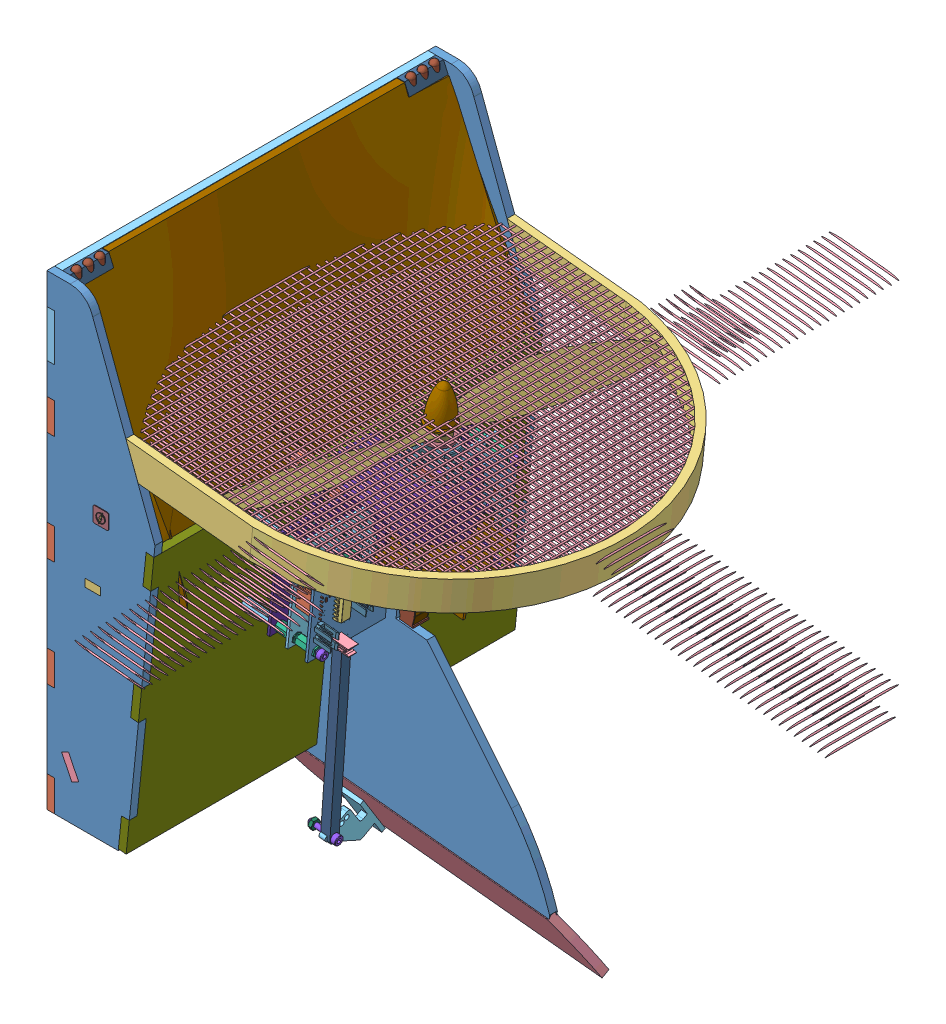
SolidWorks assembly AssTotaleSimu8, configuration Défaut. Lengths in mm. (continued)
Components (placement in the parent): (continued)
- AssStructSimu-1: AssStructSimu [Défaut] at (-125.7658 -1.8483 624.6548) x (1 0 0) z (0 0 -1) size (253.25 324.59 251.6) (continued)
  - AssCarte-1: AssCarte [Défaut] at (-42.8534 32.2132 302.028) x (-0.101852 0.9948 0) z (0.9948 0.101852 0) size (67.15 130.57 98.45) (continued)
    - carte_onduleur_v4-1: carte_onduleur_v4 [Défaut] at (-25.7639 0.8332 112.9379) size (66.52 130.57 82.34) (continued)
      - CARTE_CMD-1: CARTE_CMD [Défaut] at (25 57.2 0.803) size (60.1 130 26.71) (continued)
        - Open CASCADE STEP translator 6.8 1.20.1-1: Open CASCADE STEP translator 6.8 1.20.1 [Défaut] at origin size (60.1 130 26.71) (continued)
          - Body_1_4-1: Body_1_4 [Défaut] at (-55 5 12) size (60.1 130 26.71) (continued)
            - 175-1: 175 [Défaut] at (10 -21.7 0.803) x (0 -1 0) z (0 0 1) size (15 25.4 12.78) (continued)
              - =_[0_1_1_72]-1: =_[0_1_1_72] [Défaut] at origin size (15 25.4 12.78) (continued)
                - 173-1: 173 [Défaut] at (-1.4 -1 12) x (-1 0 0) z (0 1 0) size (15 12.78 25.4) (continued)
                  - RESC-0603_5-3: RESC-0603_5 [Défaut] at (-6.85 0 17.55) x (1 0 0) z (0 1 0) size (1.7 0.9 0.55) (continued)
                    - 152-1: 152 [Défaut] at origin (continued)
                      - =_[0_1_1_110]-1: =_[0_1_1_110] [Défaut] at origin
                      - =_[0_1_1_111]-1: =_[0_1_1_111] [Défaut] at origin
                      - =_[0_1_1_112]-1: =_[0_1_1_112] [Défaut] at origin
                      - =_[0_1_1_113]-1: =_[0_1_1_113] [Défaut] at origin
                      - =_[0_1_1_114]-1: =_[0_1_1_114] [Défaut] at origin
                      - =_[0_1_1_115]-1: =_[0_1_1_115] [Défaut] at origin
                  - RESC-0603_5-4: RESC-0603_5 [Défaut] at (-6.85 0 16.05) x (1 0 0) z (0 1 0) size (1.7 0.9 0.55)
                    - 143-1: 143 [Défaut] at origin size (1.7 0.9 0.55)
                      - =_[0_1_1_103]-1: =_[0_1_1_103] [Défaut] at origin size (0.4 0.9 0.53)
                      - =_[0_1_1_105]-1: =_[0_1_1_105] [Défaut] at origin size (0.4 0.9 0.53)
                      - =_[0_1_1_106]-1: =_[0_1_1_106] [Défaut] at origin size (1.64 0.9 0.52)
                    - 152-1: 152 [Défaut] at origin
                      - =_[0_1_1_107]-1: =_[0_1_1_107] [Défaut] at origin
                      - =_[0_1_1_109]-1: =_[0_1_1_109] [Défaut] at origin
                      - =_[0_1_1_110]-1: =_[0_1_1_110] [Défaut] at origin
                      - =_[0_1_1_111]-1: =_[0_1_1_111] [Défaut] at origin
                      - =_[0_1_1_112]-1: =_[0_1_1_112] [Défaut] at origin
                      - =_[0_1_1_113]-1: =_[0_1_1_113] [Défaut] at origin
                      - =_[0_1_1_114]-1: =_[0_1_1_114] [Défaut] at origin
                      - =_[0_1_1_115]-1: =_[0_1_1_115] [Défaut] at origin
                  - RESC-0603_5-5: RESC-0603_5 [Défaut] at (-6.85 0 5.95) x (1 0 0) z (0 1 0) size (1.7 0.9 0.55)
                    - 143-1: 143 [Défaut] at origin size (1.7 0.9 0.55)
                      - =_[0_1_1_103]-1: =_[0_1_1_103] [Défaut] at origin size (0.4 0.9 0.53)
                      - =_[0_1_1_105]-1: =_[0_1_1_105] [Défaut] at origin size (0.4 0.9 0.53)
                      - =_[0_1_1_106]-1: =_[0_1_1_106] [Défaut] at origin size (1.64 0.9 0.52)
                    - 152-1: 152 [Défaut] at origin
                      - =_[0_1_1_107]-1: =_[0_1_1_107] [Défaut] at origin
                      - =_[0_1_1_109]-1: =_[0_1_1_109] [Défaut] at origin
                      - =_[0_1_1_110]-1: =_[0_1_1_110] [Défaut] at origin
                      - =_[0_1_1_111]-1: =_[0_1_1_111] [Défaut] at origin
                      - =_[0_1_1_112]-1: =_[0_1_1_112] [Défaut] at origin
                      - =_[0_1_1_113]-1: =_[0_1_1_113] [Défaut] at origin
                      - =_[0_1_1_114]-1: =_[0_1_1_114] [Défaut] at origin
                      - =_[0_1_1_115]-1: =_[0_1_1_115] [Défaut] at origin
                  - CAPC-0603-T0.9-BN_5-1: CAPC-0603-T0.9-BN_5 [Défaut] at (-9.85 0 8.95) x (1 0 0) z (0 1 0) size (1.7 0.9 0.9)
                    - =_[0_1_1_117]-1: =_[0_1_1_117] [Défaut] at origin size (1.7 0.9 0.9)
                    - 167-1: 167 [Défaut] at origin
                      - =_[0_1_1_118]-1: =_[0_1_1_118] [Défaut] at origin
                      - =_[0_1_1_120]-1: =_[0_1_1_120] [Défaut] at origin
                      - =_[0_1_1_121]-1: =_[0_1_1_121] [Défaut] at origin
                      - =_[0_1_1_122]-1: =_[0_1_1_122] [Défaut] at origin
                      - =_[0_1_1_123]-1: =_[0_1_1_123] [Défaut] at origin
                      - =_[0_1_1_124]-1: =_[0_1_1_124] [Défaut] at origin
                      - =_[0_1_1_125]-1: =_[0_1_1_125] [Défaut] at origin
                      - =_[0_1_1_126]-1: =_[0_1_1_126] [Défaut] at origin
                  - CAPC-0603-T0.9-BN_5-2: CAPC-0603-T0.9-BN_5 [Défaut] at (-6.85 0 8.95) x (1 0 0) z (0 1 0) size (1.7 0.9 0.9)
                    - =_[0_1_1_117]-1: =_[0_1_1_117] [Défaut] at origin size (1.7 0.9 0.9)
                    - 167-1: 167 [Défaut] at origin
                      - =_[0_1_1_118]-1: =_[0_1_1_118] [Défaut] at origin
                      - =_[0_1_1_120]-1: =_[0_1_1_120] [Défaut] at origin
                      - =_[0_1_1_121]-1: =_[0_1_1_121] [Défaut] at origin
                      - =_[0_1_1_122]-1: =_[0_1_1_122] [Défaut] at origin
                      - =_[0_1_1_123]-1: =_[0_1_1_123] [Défaut] at origin
                      - =_[0_1_1_124]-1: =_[0_1_1_124] [Défaut] at origin
                      - =_[0_1_1_125]-1: =_[0_1_1_125] [Défaut] at origin
                      - =_[0_1_1_126]-1: =_[0_1_1_126] [Défaut] at origin
                  - CAPC-0603-T0.9-BN_5-3: CAPC-0603-T0.9-BN_5 [Défaut] at (-6.85 0 19.05) x (1 0 0) z (0 1 0) size (1.7 0.9 0.9)
                    - =_[0_1_1_117]-1: =_[0_1_1_117] [Défaut] at origin size (1.7 0.9 0.9)
                    - 167-1: 167 [Défaut] at origin
                      - =_[0_1_1_118]-1: =_[0_1_1_118] [Défaut] at origin
                      - =_[0_1_1_120]-1: =_[0_1_1_120] [Défaut] at origin
                      - =_[0_1_1_121]-1: =_[0_1_1_121] [Défaut] at origin
                      - =_[0_1_1_122]-1: =_[0_1_1_122] [Défaut] at origin
                      - =_[0_1_1_123]-1: =_[0_1_1_123] [Défaut] at origin
                      - =_[0_1_1_124]-1: =_[0_1_1_124] [Défaut] at origin
                      - =_[0_1_1_125]-1: =_[0_1_1_125] [Défaut] at origin
                      - =_[0_1_1_126]-1: =_[0_1_1_126] [Défaut] at origin
                  - CAPC-0603-T0.9-BN_5-4: CAPC-0603-T0.9-BN_5 [Défaut] at (-9.85 0 7.45) x (1 0 0) z (0 1 0) size (1.7 0.9 0.9)
                    - =_[0_1_1_117]-1: =_[0_1_1_117] [Défaut] at origin size (1.7 0.9 0.9)
                    - 167-1: 167 [Défaut] at origin
                      - =_[0_1_1_118]-1: =_[0_1_1_118] [Défaut] at origin
                      - =_[0_1_1_120]-1: =_[0_1_1_120] [Défaut] at origin
                      - =_[0_1_1_121]-1: =_[0_1_1_121] [Défaut] at origin
                      - =_[0_1_1_122]-1: =_[0_1_1_122] [Défaut] at origin
                      - =_[0_1_1_123]-1: =_[0_1_1_123] [Défaut] at origin
                      - =_[0_1_1_124]-1: =_[0_1_1_124] [Défaut] at origin
                      - =_[0_1_1_125]-1: =_[0_1_1_125] [Défaut] at origin
                      - =_[0_1_1_126]-1: =_[0_1_1_126] [Défaut] at origin
                  - CAPC-0603-T0.9-BN_5-5: CAPC-0603-T0.9-BN_5 [Défaut] at (-9.85 0 17.55) x (1 0 0) z (0 1 0) size (1.7 0.9 0.9)
                    - =_[0_1_1_117]-1: =_[0_1_1_117] [Défaut] at origin size (1.7 0.9 0.9)
                    - 167-1: 167 [Défaut] at origin
                      - =_[0_1_1_118]-1: =_[0_1_1_118] [Défaut] at origin
                      - =_[0_1_1_120]-1: =_[0_1_1_120] [Défaut] at origin
                      - =_[0_1_1_121]-1: =_[0_1_1_121] [Défaut] at origin
                      - =_[0_1_1_122]-1: =_[0_1_1_122] [Défaut] at origin
                      - =_[0_1_1_123]-1: =_[0_1_1_123] [Défaut] at origin
                      - =_[0_1_1_124]-1: =_[0_1_1_124] [Défaut] at origin
                      - =_[0_1_1_125]-1: =_[0_1_1_125] [Défaut] at origin
                      - =_[0_1_1_126]-1: =_[0_1_1_126] [Défaut] at origin
            - 177-1: 177 [Défaut] at (52.1 -16.5 -0.803) x (1 0 0) z (0 0 -1) size (2.34 1.04 0.5)
              - =_[0_1_1_30]-1: =_[0_1_1_30] [Défaut] at origin size (2.34 1.04 0.5)
                - 32_2-1: 32_2 [Défaut] at origin size (2.29 1.04 0.43)
                - 33_2-1: 33_2 [Défaut] at (0.3048 0 0) x (-1 0 0) z (0 0 1) size (0.51 1.02 0.5)
                - 34-1: 34 [Défaut] at origin size (0.51 1.02 0.5)
            - 179-1: 179 [Défaut] at (22.5336 -121.5 -0.803) x (-1 0 0) z (0 0 -1) size (2.34 1.04 0.5)
              - =_[0_1_1_30]-1: =_[0_1_1_30] [Défaut] at origin size (2.34 1.04 0.5)
                - 32_2-1: 32_2 [Défaut] at origin size (2.29 1.04 0.43)
                - 33_2-1: 33_2 [Défaut] at (0.3048 0 0) x (-1 0 0) z (0 0 1) size (0.51 1.02 0.5)
                - 34-1: 34 [Défaut] at origin size (0.51 1.02 0.5)
            - 181-1: 181 [Défaut] at (48.6 -127 -0.803) x (-1 0 0) z (0 0 -1) size (2.34 1.04 0.5)
              - =_[0_1_1_30]-1: =_[0_1_1_30] [Défaut] at origin size (2.34 1.04 0.5)
                - 32_2-1: 32_2 [Défaut] at origin size (2.29 1.04 0.43)
                - 33_2-1: 33_2 [Défaut] at (0.3048 0 0) x (-1 0 0) z (0 0 1) size (0.51 1.02 0.5)
                - 34-1: 34 [Défaut] at origin size (0.51 1.02 0.5)
            - 183-1: 183 [Défaut] at (26.0189 -121.5 0.803) size (2.34 1.04 0.5)
              - =_[0_1_1_30]-1: =_[0_1_1_30] [Défaut] at origin size (2.34 1.04 0.5)
                - 32_2-1: 32_2 [Défaut] at origin size (2.29 1.04 0.43)
                - 33_2-1: 33_2 [Défaut] at (0.3048 0 0) x (-1 0 0) z (0 0 1) size (0.51 1.02 0.5)
                - 34-1: 34 [Défaut] at origin size (0.51 1.02 0.5)
            - 185-1: 185 [Défaut] at (30.3664 -19 -0.803) x (1 0 0) z (0 0 -1) size (2.34 1.04 0.5)
              - =_[0_1_1_30]-1: =_[0_1_1_30] [Défaut] at origin size (2.34 1.04 0.5)
                - 32_2-1: 32_2 [Défaut] at origin size (2.29 1.04 0.43)
                - 33_2-1: 33_2 [Défaut] at (0.3048 0 0) x (-1 0 0) z (0 0 1) size (0.51 1.02 0.5)
                - 34-1: 34 [Défaut] at origin size (0.51 1.02 0.5)
            - 187-1: 187 [Défaut] at (51.7 -114.3 -0.803) x (0 1 0) z (0 0 -1) size (2.34 1.04 0.5)
              - =_[0_1_1_30]-1: =_[0_1_1_30] [Défaut] at origin size (2.34 1.04 0.5)
                - 32_2-1: 32_2 [Défaut] at origin size (2.29 1.04 0.43)
                - 33_2-1: 33_2 [Défaut] at (0.3048 0 0) x (-1 0 0) z (0 0 1) size (0.51 1.02 0.5)
                - 34-1: 34 [Défaut] at origin size (0.51 1.02 0.5)
            - 189-1: 189 [Défaut] at (50 -114.3 -0.803) x (0 1 0) z (0 0 -1) size (2.34 1.04 0.5)
              - =_[0_1_1_30]-1: =_[0_1_1_30] [Défaut] at origin size (2.34 1.04 0.5)
                - 32_2-1: 32_2 [Défaut] at origin size (2.29 1.04 0.43)
                - 33_2-1: 33_2 [Défaut] at (0.3048 0 0) x (-1 0 0) z (0 0 1) size (0.51 1.02 0.5)
                - 34-1: 34 [Défaut] at origin size (0.51 1.02 0.5)
            - 192-1: 192 [Défaut] at (37.94 -103.3308 0.803) x (-1 0 0) z (0 0 1) size (5.08 5 14.3)
              - =_[0_1_1_135]-1: =_[0_1_1_135] [Défaut] at origin size (5.08 5 14.3)
                - 190-1: 190 [Défaut] at (1.2 0 11) size (5.08 5 14.3)
            - 194-1: 194 [Défaut] at (32.7796 -102.6 -0.803) x (-1 0 0) z (0 0 -1) size (2.54 1.98 0.64)
              - =_[0_1_1_46]-1: =_[0_1_1_46] [Défaut] at origin size (2.54 1.98 0.64)
                - 52-1: 52 [Défaut] at origin size (2.54 1.14 0.58)
                - 53-1: 53 [Défaut] x (0 -1 0) z (0 0 1) size (0.43 0.51 0.38)
                - 54-1: 54 [Défaut] at (1.8796 1.8796 0) x (0 -1 0) z (0 0 1) size (0.43 0.51 0.38)
                - 55-1: 55 [Défaut] at (-0.9652 -2.8448 0) x (0 1 0) z (0 0 1) size (0.41 0.51 0.38)
            - 196-1: 196 [Défaut] at (40.243 -104.3176 -0.803) x (0 1 0) z (0 0 -1) size (2.34 1.04 0.5)
              - =_[0_1_1_30]-1: =_[0_1_1_30] [Défaut] at origin size (2.34 1.04 0.5)
                - 32_2-1: 32_2 [Défaut] at origin size (2.29 1.04 0.43)
                - 33_2-1: 33_2 [Défaut] at (0.3048 0 0) x (-1 0 0) z (0 0 1) size (0.51 1.02 0.5)
                - 34-1: 34 [Défaut] at origin size (0.51 1.02 0.5)
            - 198-1: 198 [Défaut] at (42 -104.3176 -0.803) x (0 1 0) z (0 0 -1) size (2.34 1.04 0.5)
              - =_[0_1_1_30]-1: =_[0_1_1_30] [Défaut] at origin size (2.34 1.04 0.5)
                - 32_2-1: 32_2 [Défaut] at origin size (2.29 1.04 0.43)
                - 33_2-1: 33_2 [Défaut] at (0.3048 0 0) x (-1 0 0) z (0 0 1) size (0.51 1.02 0.5)
                - 34-1: 34 [Défaut] at origin size (0.51 1.02 0.5)
            - 200-1: 200 [Défaut] at (30.1 -112.9336 -0.803) x (0 1 0) z (0 0 -1) size (2.34 1.04 0.5)
              - =_[0_1_1_30]-1: =_[0_1_1_30] [Défaut] at origin size (2.34 1.04 0.5)
                - 32_2-1: 32_2 [Défaut] at origin size (2.29 1.04 0.43)
                - 33_2-1: 33_2 [Défaut] at (0.3048 0 0) x (-1 0 0) z (0 0 1) size (0.51 1.02 0.5)
                - 34-1: 34 [Défaut] at origin size (0.51 1.02 0.5)
      - C2_1-1: C2_1 [Défaut] at (-20.6984 1.8 -0.803) x (1 0 0) z (0 0 -1) size (2.34 1.04 0.5)
        - Open CASCADE STEP translator 6.8 1.6.1-1: Open CASCADE STEP translator 6.8 1.6.1 [Défaut] at origin size (2.34 1.04 0.5)
          - Body_1-1: Body_1 [Défaut] at origin size (2.29 1.04 0.43)
          - Pin_1-1: Pin_1 [Défaut] at (0.3048 0 0) x (-1 0 0) z (0 0 1) size (0.51 1.02 0.5)
          - Pin_2-1: Pin_2 [Défaut] at origin size (0.51 1.02 0.5)
      - C2_2-1: C2_2 [Défaut] at (-24.2 1.8 -0.803) x (1 0 0) z (0 0 -1) size (2.34 1.04 0.5)
        - Open CASCADE STEP translator 6.8 1.6.1-1: Open CASCADE STEP translator 6.8 1.6.1 [Défaut] at origin size (2.34 1.04 0.5)
          - Body_1-1: Body_1 [Défaut] at origin size (2.29 1.04 0.43)
          - Pin_1-1: Pin_1 [Défaut] at (0.3048 0 0) x (-1 0 0) z (0 0 1) size (0.51 1.02 0.5)
          - Pin_2-1: Pin_2 [Défaut] at origin size (0.51 1.02 0.5)
      - C3_1-1: C3_1 [Défaut] at (-20.9176 -12.8 -0.803) x (1 0 0) z (0 0 -1) size (2.34 1.04 0.5)
        - Open CASCADE STEP translator 6.8 1.6.1-1: Open CASCADE STEP translator 6.8 1.6.1 [Défaut] at origin size (2.34 1.04 0.5)
          - Body_1-1: Body_1 [Défaut] at origin size (2.29 1.04 0.43)
          - Pin_1-1: Pin_1 [Défaut] at (0.3048 0 0) x (-1 0 0) z (0 0 1) size (0.51 1.02 0.5)
          - Pin_2-1: Pin_2 [Défaut] at origin size (0.51 1.02 0.5)
      - C3_2-1: C3_2 [Défaut] at (-24.4 -12.8 -0.803) x (1 0 0) z (0 0 -1) size (2.34 1.04 0.5)
        - Open CASCADE STEP translator 6.8 1.6.1-1: Open CASCADE STEP translator 6.8 1.6.1 [Défaut] at origin size (2.34 1.04 0.5)
          - Body_1-1: Body_1 [Défaut] at origin size (2.29 1.04 0.43)
          - Pin_1-1: Pin_1 [Défaut] at (0.3048 0 0) x (-1 0 0) z (0 0 1) size (0.51 1.02 0.5)
          - Pin_2-1: Pin_2 [Défaut] at origin size (0.51 1.02 0.5)
      - D_CUR-1: D_CUR [Défaut] at (-12.4432 3.85 -0.803) x (0 -1 0) z (0 0 -1) size (2.7 5.2 1.11)
        - Open CASCADE STEP translator 6.8 1.25.1-1: Open CASCADE STEP translator 6.8 1.25.1 [Défaut] at origin size (2.7 5.2 1.11)
          - Body_1_5-1: Body_1_5 [Défaut] at (1.2 -4 0) x (0 1 0) z (0 0 1) size (5.2 2.7 1.11)
            - =_[0_1_1_3]_4-1: =_[0_1_1_3]_4 [Défaut] at origin size (0.39 0.64 0.01)
            - =_[0_1_1_4]_4-1: =_[0_1_1_4]_4 [Défaut] at origin size (0.6 1.9 0.2)
            - =_[0_1_1_5]_4-1: =_[0_1_1_5]_4 [Défaut] at origin size (0.21 0.08 0.01)
            - =_[0_1_1_6]_2-1: =_[0_1_1_6]_2 [Défaut] at origin size (0.6 1.9 0.2)
            - =_[0_1_1_7]_2-1: =_[0_1_1_7]_2 [Défaut] at origin size (0.46 0.68 0.01)
            - =_[0_1_1_8]_2-1: =_[0_1_1_8]_2 [Défaut] at origin size (0.38 0.66 0.01)
            - =_[0_1_1_9]-1: =_[0_1_1_9] [Défaut] at origin size (0.2 0.62 0.01)
            - =_[0_1_1_10]-1: =_[0_1_1_10] [Défaut] at origin size (4 2.7 1.1)
            - =_[0_1_1_11]-1: =_[0_1_1_11] [Défaut] at origin size (0.46 0.63 0.01)
            - =_[0_1_1_12]-1: =_[0_1_1_12] [Défaut] at origin size (0.56 0.68 0.01)
      - RC1_1-1: RC1_1 [Défaut] at (-20.7176 8.1 -0.803) x (1 0 0) z (0 0 -1) size (2.34 1.04 0.5)
        - Open CASCADE STEP translator 6.8 1.12.1-1: Open CASCADE STEP translator 6.8 1.12.1 [Défaut] at origin size (2.34 1.04 0.5)
          - Body_1_3-1: Body_1_3 [Défaut] at origin size (2.29 1.04 0.43)
          - Pin_1_2-1: Pin_1_2 [Défaut] at (0.3048 0 0) x (-1 0 0) z (0 0 1) size (0.51 1.02 0.5)
          - Pin_2_2-1: Pin_2_2 [Défaut] at origin size (0.51 1.02 0.5)
      - RC1_2-1: RC1_2 [Défaut] at (-22 8.1 -0.803) x (-1 0 0) z (0 0 -1) size (2.34 1.04 0.5)
        - Open CASCADE STEP translator 6.8 1.12.1-1: Open CASCADE STEP translator 6.8 1.12.1 [Défaut] at origin size (2.34 1.04 0.5)
          - Body_1_3-1: Body_1_3 [Défaut] at origin size (2.29 1.04 0.43)
          - Pin_1_2-1: Pin_1_2 [Défaut] at (0.3048 0 0) x (-1 0 0) z (0 0 1) size (0.51 1.02 0.5)
          - Pin_2_2-1: Pin_2_2 [Défaut] at origin size (0.51 1.02 0.5)
      - RC2_1-1: RC2_1 [Défaut] at (-20.716 0.243 -0.803) x (1 0 0) z (0 0 -1) size (2.34 1.04 0.5)
        - Open CASCADE STEP translator 6.8 1.12.1-1: Open CASCADE STEP translator 6.8 1.12.1 [Défaut] at origin size (2.34 1.04 0.5)
          - Body_1_3-1: Body_1_3 [Défaut] at origin size (2.29 1.04 0.43)
          - Pin_1_2-1: Pin_1_2 [Défaut] at (0.3048 0 0) x (-1 0 0) z (0 0 1) size (0.51 1.02 0.5)
          - Pin_2_2-1: Pin_2_2 [Défaut] at origin size (0.51 1.02 0.5)
      - RC2_2-1: RC2_2 [Défaut] at (-22 0.18 -0.803) x (-1 0 0) z (0 0 -1) size (2.34 1.04 0.5)
        - Open CASCADE STEP translator 6.8 1.12.1-1: Open CASCADE STEP translator 6.8 1.12.1 [Défaut] at origin size (2.34 1.04 0.5)
          - Body_1_3-1: Body_1_3 [Défaut] at origin size (2.29 1.04 0.43)
          - Pin_1_2-1: Pin_1_2 [Défaut] at (0.3048 0 0) x (-1 0 0) z (0 0 1) size (0.51 1.02 0.5)
          - Pin_2_2-1: Pin_2_2 [Défaut] at origin size (0.51 1.02 0.5)
      - RC3_1-1: RC3_1 [Défaut] at (-20.9336 -14.5 -0.803) x (1 0 0) z (0 0 -1) size (2.34 1.04 0.5)
        - Open CASCADE STEP translator 6.8 1.12.1-1: Open CASCADE STEP translator 6.8 1.12.1 [Défaut] at origin size (2.34 1.04 0.5)
          - Body_1_3-1: Body_1_3 [Défaut] at origin size (2.29 1.04 0.43)
          - Pin_1_2-1: Pin_1_2 [Défaut] at (0.3048 0 0) x (-1 0 0) z (0 0 1) size (0.51 1.02 0.5)
          - Pin_2_2-1: Pin_2_2 [Défaut] at origin size (0.51 1.02 0.5)
      - RC3_2-1: RC3_2 [Défaut] at (-22.3 -14.5 -0.803) x (-1 0 0) z (0 0 -1) size (2.34 1.04 0.5)
        - Open CASCADE STEP translator 6.8 1.12.1-1: Open CASCADE STEP translator 6.8 1.12.1 [Défaut] at origin size (2.34 1.04 0.5)
          - Body_1_3-1: Body_1_3 [Défaut] at origin size (2.29 1.04 0.43)
          - Pin_1_2-1: Pin_1_2 [Défaut] at (0.3048 0 0) x (-1 0 0) z (0 0 1) size (0.51 1.02 0.5)
          - Pin_2_2-1: Pin_2_2 [Défaut] at origin size (0.51 1.02 0.5)
      - U_MES_CUR-1: U_MES_CUR [Défaut] at (-11.5 6.7816 0.803) size (2.54 2.41 0.76)
        - Open CASCADE STEP translator 6.8 1.32.1-1: Open CASCADE STEP translator 6.8 1.32.1 [Défaut] at origin size (2.54 2.41 0.76)
          - Body_1_5-1: Body_1_5 [Défaut] at origin size (2.54 1.27 0.71)
          - Pin_1_3-1: Pin_1_3 [Défaut] at (-2.1082 0.2286 0) x (0 -1 0) z (0 0 1) size (1.14 0.25 0.47)
          - Pin_2_3-1: Pin_2_3 [Défaut] at (-0.2032 2.1336 0) x (0 -1 0) z (0 0 1) size (1.14 0.25 0.47)
      - COMP1-1: COMP1 [Défaut] at (-16.3 -36.2 0.803) x (-1 0 0) z (0 0 1) size (2.03 1.88 0.51)
        - Open CASCADE STEP translator 6.8 1.33.1-1: Open CASCADE STEP translator 6.8 1.33.1 [Défaut] at origin size (2.03 1.88 0.51)
          - Body_1_6-1: Body_1_6 [Défaut] at origin size (2.03 1.02 0.46)
          - Pin_1_4-1: Pin_1_4 [Défaut] x (0 1 0) z (0 0 1) size (0.45 0.25 0.32)
          - Pin_2_4-1: Pin_2_4 [Défaut] at (0.65 -0.65 0) x (0 1 0) z (0 0 1) size (0.45 0.25 0.32)
          - Pin_3-1: Pin_3 [Défaut] at (1.3 -1.3 0) x (0 1 0) z (0 0 1) size (0.45 0.25 0.32)
          - Pin_4-1: Pin_4 [Défaut] at (-0.5 3.1 0) x (0 -1 0) z (0 0 1) size (0.41 0.25 0.32)
          - Pin_5-1: Pin_5 [Défaut] at (-1.8 1.8 0) x (0 -1 0) z (0 0 1) size (0.41 0.25 0.32)
      - COMP2-1: COMP2 [Défaut] at (-14.3 -9.6 0.803) x (-1 0 0) z (0 0 1) size (2.03 1.88 0.51)
        - Open CASCADE STEP translator 6.8 1.33.1-1: Open CASCADE STEP translator 6.8 1.33.1 [Défaut] at origin size (2.03 1.88 0.51)
          - Body_1_6-1: Body_1_6 [Défaut] at origin size (2.03 1.02 0.46)
          - Pin_1_4-1: Pin_1_4 [Défaut] x (0 1 0) z (0 0 1) size (0.45 0.25 0.32)
          - Pin_2_4-1: Pin_2_4 [Défaut] at (0.65 -0.65 0) x (0 1 0) z (0 0 1) size (0.45 0.25 0.32)
          - Pin_3-1: Pin_3 [Défaut] at (1.3 -1.3 0) x (0 1 0) z (0 0 1) size (0.45 0.25 0.32)
          - Pin_4-1: Pin_4 [Défaut] at (-0.5 3.1 0) x (0 -1 0) z (0 0 1) size (0.41 0.25 0.32)
          - Pin_5-1: Pin_5 [Défaut] at (-1.8 1.8 0) x (0 -1 0) z (0 0 1) size (0.41 0.25 0.32)
      - COMP3-1: COMP3 [Défaut] at (-15.9 -23.2 0.803) x (-1 0 0) z (0 0 1) size (2.03 1.88 0.51)
        - Open CASCADE STEP translator 6.8 1.33.1-1: Open CASCADE STEP translator 6.8 1.33.1 [Défaut] at origin size (2.03 1.88 0.51)
          - Body_1_6-1: Body_1_6 [Défaut] at origin size (2.03 1.02 0.46)
          - Pin_1_4-1: Pin_1_4 [Défaut] x (0 1 0) z (0 0 1) size (0.45 0.25 0.32)
          - Pin_2_4-1: Pin_2_4 [Défaut] at (0.65 -0.65 0) x (0 1 0) z (0 0 1) size (0.45 0.25 0.32)
          - Pin_3-1: Pin_3 [Défaut] at (1.3 -1.3 0) x (0 1 0) z (0 0 1) size (0.45 0.25 0.32)
          - Pin_4-1: Pin_4 [Défaut] at (-0.5 3.1 0) x (0 -1 0) z (0 0 1) size (0.41 0.25 0.32)
          - Pin_5-1: Pin_5 [Défaut] at (-1.8 1.8 0) x (0 -1 0) z (0 0 1) size (0.41 0.25 0.32)
      - CP1-1: CP1 [Défaut] at (-18.9 -38.2 0.803) x (0 1 0) z (0 0 1) size (2.34 1.04 0.5)
        - Open CASCADE STEP translator 6.8 1.6.1-1: Open CASCADE STEP translator 6.8 1.6.1 [Défaut] at origin size (2.34 1.04 0.5)
          - Body_1-1: Body_1 [Défaut] at origin size (2.29 1.04 0.43)
          - Pin_1-1: Pin_1 [Défaut] at (0.3048 0 0) x (-1 0 0) z (0 0 1) size (0.51 1.02 0.5)
          - Pin_2-1: Pin_2 [Défaut] at origin size (0.51 1.02 0.5)
      - CP2-1: CP2 [Défaut] at (-16.9 -11.6 0.803) x (0 1 0) z (0 0 1) size (2.34 1.04 0.5)
        - Open CASCADE STEP translator 6.8 1.6.1-1: Open CASCADE STEP translator 6.8 1.6.1 [Défaut] at origin size (2.34 1.04 0.5)
          - Body_1-1: Body_1 [Défaut] at origin size (2.29 1.04 0.43)
          - Pin_1-1: Pin_1 [Défaut] at (0.3048 0 0) x (-1 0 0) z (0 0 1) size (0.51 1.02 0.5)
          - Pin_2-1: Pin_2 [Défaut] at origin size (0.51 1.02 0.5)
      - CP3-1: CP3 [Défaut] at (-18.5 -25.2 0.803) x (0 1 0) z (0 0 1) size (2.34 1.04 0.5)
        - Open CASCADE STEP translator 6.8 1.6.1-1: Open CASCADE STEP translator 6.8 1.6.1 [Défaut] at origin size (2.34 1.04 0.5)
          - Body_1-1: Body_1 [Défaut] at origin size (2.29 1.04 0.43)
          - Pin_1-1: Pin_1 [Défaut] at (0.3048 0 0) x (-1 0 0) z (0 0 1) size (0.51 1.02 0.5)
          - Pin_2-1: Pin_2 [Défaut] at origin size (0.51 1.02 0.5)
      - C_DEC_COM1-1: C_DEC_COM1 [Défaut] at (-15 -36 0.803) x (0 -1 0) z (0 0 1) size (2.34 1.04 0.5)
        - Open CASCADE STEP translator 6.8 1.6.1-1: Open CASCADE STEP translator 6.8 1.6.1 [Défaut] at origin size (2.34 1.04 0.5)
          - Body_1-1: Body_1 [Défaut] at origin size (2.29 1.04 0.43)
          - Pin_1-1: Pin_1 [Défaut] at (0.3048 0 0) x (-1 0 0) z (0 0 1) size (0.51 1.02 0.5)
          - Pin_2-1: Pin_2 [Défaut] at origin size (0.51 1.02 0.5)
      - C_DEC_COMP2-1: C_DEC_COMP2 [Défaut] at (-13 -9.3 0.803) x (0 -1 0) z (0 0 1) size (2.34 1.04 0.5)
        - Open CASCADE STEP translator 6.8 1.6.1-1: Open CASCADE STEP translator 6.8 1.6.1 [Défaut] at origin size (2.34 1.04 0.5)
          - Body_1-1: Body_1 [Défaut] at origin size (2.29 1.04 0.43)
          - Pin_1-1: Pin_1 [Défaut] at (0.3048 0 0) x (-1 0 0) z (0 0 1) size (0.51 1.02 0.5)
          - Pin_2-1: Pin_2 [Défaut] at origin size (0.51 1.02 0.5)
      - C_DEC_COMP3-1: C_DEC_COMP3 [Défaut] at (-14.6 -22.9 0.803) x (0 -1 0) z (0 0 1) size (2.34 1.04 0.5)
        - Open CASCADE STEP translator 6.8 1.6.1-1: Open CASCADE STEP translator 6.8 1.6.1 [Défaut] at origin size (2.34 1.04 0.5)
          - Body_1-1: Body_1 [Défaut] at origin size (2.29 1.04 0.43)
          - Pin_1-1: Pin_1 [Défaut] at (0.3048 0 0) x (-1 0 0) z (0 0 1) size (0.51 1.02 0.5)
          - Pin_2-1: Pin_2 [Défaut] at origin size (0.51 1.02 0.5)
      - D_VBAT-1: D_VBAT [Défaut] at (-1.2 46.4 0.803) x (0 -1 0) z (0 0 1) size (2.34 1.04 0.5)
        - Open CASCADE STEP translator 6.8 1.6.1-1: Open CASCADE STEP translator 6.8 1.6.1 [Défaut] at origin size (2.34 1.04 0.5)
          - Body_1-1: Body_1 [Défaut] at origin size (2.29 1.04 0.43)
          - Pin_1-1: Pin_1 [Défaut] at (0.3048 0 0) x (-1 0 0) z (0 0 1) size (0.51 1.02 0.5)
          - Pin_2-1: Pin_2 [Défaut] at origin size (0.51 1.02 0.5)
      - D_3V-1: D_3V [Défaut] at (1.3 46.3 0.803) x (0 -1 0) z (0 0 1) size (2.34 1.04 0.5)
        - Open CASCADE STEP translator 6.8 1.6.1-1: Open CASCADE STEP translator 6.8 1.6.1 [Défaut] at origin size (2.34 1.04 0.5)
          - Body_1-1: Body_1 [Défaut] at origin size (2.29 1.04 0.43)
          - Pin_1-1: Pin_1 [Défaut] at (0.3048 0 0) x (-1 0 0) z (0 0 1) size (0.51 1.02 0.5)
          - Pin_2-1: Pin_2 [Défaut] at origin size (0.51 1.02 0.5)
      - D_5V-1: D_5V [Défaut] at (-3.7 46.4 0.803) x (0 -1 0) z (0 0 1) size (2.34 1.04 0.5)
        - Open CASCADE STEP translator 6.8 1.6.1-1: Open CASCADE STEP translator 6.8 1.6.1 [Défaut] at origin size (2.34 1.04 0.5)
          - Body_1-1: Body_1 [Défaut] at origin size (2.29 1.04 0.43)
          - Pin_1-1: Pin_1 [Défaut] at (0.3048 0 0) x (-1 0 0) z (0 0 1) size (0.51 1.02 0.5)
          - Pin_2-1: Pin_2 [Défaut] at origin size (0.51 1.02 0.5)
      - R1_1-1: R1_1 [Défaut] at (-20.2 -36.1 0.803) x (-1 0 0) z (0 0 1) size (2.34 1.04 0.5)
        - Open CASCADE STEP translator 6.8 1.12.1-1: Open CASCADE STEP translator 6.8 1.12.1 [Défaut] at origin size (2.34 1.04 0.5)
          - Body_1_3-1: Body_1_3 [Défaut] at origin size (2.29 1.04 0.43)
          - Pin_1_2-1: Pin_1_2 [Défaut] at (0.3048 0 0) x (-1 0 0) z (0 0 1) size (0.51 1.02 0.5)
          - Pin_2_2-1: Pin_2_2 [Défaut] at origin size (0.51 1.02 0.5)
      - R1_2-1: R1_2 [Défaut] at (-15.5 -34.6 0.803) x (-1 0 0) z (0 0 1) size (2.34 1.04 0.5)
        - Open CASCADE STEP translator 6.8 1.12.1-1: Open CASCADE STEP translator 6.8 1.12.1 [Défaut] at origin size (2.34 1.04 0.5)
          - Body_1_3-1: Body_1_3 [Défaut] at origin size (2.29 1.04 0.43)
          - Pin_1_2-1: Pin_1_2 [Défaut] at (0.3048 0 0) x (-1 0 0) z (0 0 1) size (0.51 1.02 0.5)
          - Pin_2_2-1: Pin_2_2 [Défaut] at origin size (0.51 1.02 0.5)
      - R1_3-1: R1_3 [Défaut] at (-20.3 -39.9 0.803) x (-1 0 0) z (0 0 1) size (2.34 1.04 0.5)
        - Open CASCADE STEP translator 6.8 1.12.1-1: Open CASCADE STEP translator 6.8 1.12.1 [Défaut] at origin size (2.34 1.04 0.5)
          - Body_1_3-1: Body_1_3 [Défaut] at origin size (2.29 1.04 0.43)
          - Pin_1_2-1: Pin_1_2 [Défaut] at (0.3048 0 0) x (-1 0 0) z (0 0 1) size (0.51 1.02 0.5)
          - Pin_2_2-1: Pin_2_2 [Défaut] at origin size (0.51 1.02 0.5)
      - R1_4-1: R1_4 [Défaut] at (-20.3 -38.1 0.803) x (-1 0 0) z (0 0 1) size (2.34 1.04 0.5)
        - Open CASCADE STEP translator 6.8 1.12.1-1: Open CASCADE STEP translator 6.8 1.12.1 [Défaut] at origin size (2.34 1.04 0.5)
          - Body_1_3-1: Body_1_3 [Défaut] at origin size (2.29 1.04 0.43)
          - Pin_1_2-1: Pin_1_2 [Défaut] at (0.3048 0 0) x (-1 0 0) z (0 0 1) size (0.51 1.02 0.5)
          - Pin_2_2-1: Pin_2_2 [Défaut] at origin size (0.51 1.02 0.5)
      - R1_5-1: R1_5 [Défaut] at (-17.1336 -39.7 0.803) size (2.34 1.04 0.5)
        - Open CASCADE STEP translator 6.8 1.12.1-1: Open CASCADE STEP translator 6.8 1.12.1 [Défaut] at origin size (2.34 1.04 0.5)
          - Body_1_3-1: Body_1_3 [Défaut] at origin size (2.29 1.04 0.43)
          - Pin_1_2-1: Pin_1_2 [Défaut] at (0.3048 0 0) x (-1 0 0) z (0 0 1) size (0.51 1.02 0.5)
          - Pin_2_2-1: Pin_2_2 [Défaut] at origin size (0.51 1.02 0.5)
      - R2_1-1: R2_1 [Défaut] at (-18.5 -9.5 0.803) x (-1 0 0) z (0 0 1) size (2.34 1.04 0.5)
        - Open CASCADE STEP translator 6.8 1.12.1-1: Open CASCADE STEP translator 6.8 1.12.1 [Défaut] at origin size (2.34 1.04 0.5)
          - Body_1_3-1: Body_1_3 [Défaut] at origin size (2.29 1.04 0.43)
          - Pin_1_2-1: Pin_1_2 [Défaut] at (0.3048 0 0) x (-1 0 0) z (0 0 1) size (0.51 1.02 0.5)
          - Pin_2_2-1: Pin_2_2 [Défaut] at origin size (0.51 1.02 0.5)
      - R2_2-1: R2_2 [Défaut] at (-13.1 -8 0.803) x (-1 0 0) z (0 0 1) size (2.34 1.04 0.5)
        - Open CASCADE STEP translator 6.8 1.12.1-1: Open CASCADE STEP translator 6.8 1.12.1 [Défaut] at origin size (2.34 1.04 0.5)
          - Body_1_3-1: Body_1_3 [Défaut] at origin size (2.29 1.04 0.43)
          - Pin_1_2-1: Pin_1_2 [Défaut] at (0.3048 0 0) x (-1 0 0) z (0 0 1) size (0.51 1.02 0.5)
          - Pin_2_2-1: Pin_2_2 [Défaut] at origin size (0.51 1.02 0.5)
      - R2_3-1: R2_3 [Défaut] at (-18.5 -11.2 0.803) x (-1 0 0) z (0 0 1) size (2.34 1.04 0.5)
        - Open CASCADE STEP translator 6.8 1.12.1-1: Open CASCADE STEP translator 6.8 1.12.1 [Défaut] at origin size (2.34 1.04 0.5)
          - Body_1_3-1: Body_1_3 [Défaut] at origin size (2.29 1.04 0.43)
          - Pin_1_2-1: Pin_1_2 [Défaut] at (0.3048 0 0) x (-1 0 0) z (0 0 1) size (0.51 1.02 0.5)
          - Pin_2_2-1: Pin_2_2 [Défaut] at origin size (0.51 1.02 0.5)
      - R2_4-1: R2_4 [Défaut] at (-18.5 -12.8 0.803) x (-1 0 0) z (0 0 1) size (2.34 1.04 0.5)
        - Open CASCADE STEP translator 6.8 1.12.1-1: Open CASCADE STEP translator 6.8 1.12.1 [Défaut] at origin size (2.34 1.04 0.5)
          - Body_1_3-1: Body_1_3 [Défaut] at origin size (2.29 1.04 0.43)
          - Pin_1_2-1: Pin_1_2 [Défaut] at (0.3048 0 0) x (-1 0 0) z (0 0 1) size (0.51 1.02 0.5)
          - Pin_2_2-1: Pin_2_2 [Défaut] at origin size (0.51 1.02 0.5)
      - R2_5-1: R2_5 [Défaut] at (-15.1336 -13 0.803) size (2.34 1.04 0.5)
        - Open CASCADE STEP translator 6.8 1.12.1-1: Open CASCADE STEP translator 6.8 1.12.1 [Défaut] at origin size (2.34 1.04 0.5)
          - Body_1_3-1: Body_1_3 [Défaut] at origin size (2.29 1.04 0.43)
          - Pin_1_2-1: Pin_1_2 [Défaut] at (0.3048 0 0) x (-1 0 0) z (0 0 1) size (0.51 1.02 0.5)
          - Pin_2_2-1: Pin_2_2 [Défaut] at origin size (0.51 1.02 0.5)
      - R3_1-1: R3_1 [Défaut] at (-19.9 -23.1 0.803) x (-1 0 0) z (0 0 1) size (2.34 1.04 0.5)
        - Open CASCADE STEP translator 6.8 1.12.1-1: Open CASCADE STEP translator 6.8 1.12.1 [Défaut] at origin size (2.34 1.04 0.5)
          - Body_1_3-1: Body_1_3 [Défaut] at origin size (2.29 1.04 0.43)
          - Pin_1_2-1: Pin_1_2 [Défaut] at (0.3048 0 0) x (-1 0 0) z (0 0 1) size (0.51 1.02 0.5)
          - Pin_2_2-1: Pin_2_2 [Défaut] at origin size (0.51 1.02 0.5)
      - R3_2-1: R3_2 [Défaut] at (-14.7 -21.6 0.803) x (-1 0 0) z (0 0 1) size (2.34 1.04 0.5)
        - Open CASCADE STEP translator 6.8 1.12.1-1: Open CASCADE STEP translator 6.8 1.12.1 [Défaut] at origin size (2.34 1.04 0.5)
          - Body_1_3-1: Body_1_3 [Défaut] at origin size (2.29 1.04 0.43)
          - Pin_1_2-1: Pin_1_2 [Défaut] at (0.3048 0 0) x (-1 0 0) z (0 0 1) size (0.51 1.02 0.5)
          - Pin_2_2-1: Pin_2_2 [Défaut] at origin size (0.51 1.02 0.5)
      - R3_3-1: R3_3 [Défaut] at (-19.9 -24.8 0.803) x (-1 0 0) z (0 0 1) size (2.34 1.04 0.5)
        - Open CASCADE STEP translator 6.8 1.12.1-1: Open CASCADE STEP translator 6.8 1.12.1 [Défaut] at origin size (2.34 1.04 0.5)
          - Body_1_3-1: Body_1_3 [Défaut] at origin size (2.29 1.04 0.43)
          - Pin_1_2-1: Pin_1_2 [Défaut] at (0.3048 0 0) x (-1 0 0) z (0 0 1) size (0.51 1.02 0.5)
          - Pin_2_2-1: Pin_2_2 [Défaut] at origin size (0.51 1.02 0.5)
      - R3_4-1: R3_4 [Défaut] at (-19.9 -26.4 0.803) x (-1 0 0) z (0 0 1) size (2.34 1.04 0.5)
        - Open CASCADE STEP translator 6.8 1.12.1-1: Open CASCADE STEP translator 6.8 1.12.1 [Défaut] at origin size (2.34 1.04 0.5)
          - Body_1_3-1: Body_1_3 [Défaut] at origin size (2.29 1.04 0.43)
          - Pin_1_2-1: Pin_1_2 [Défaut] at (0.3048 0 0) x (-1 0 0) z (0 0 1) size (0.51 1.02 0.5)
          - Pin_2_2-1: Pin_2_2 [Défaut] at origin size (0.51 1.02 0.5)
      - R3_5-1: R3_5 [Défaut] at (-16.7336 -26.5 0.803) size (2.34 1.04 0.5)
        - Open CASCADE STEP translator 6.8 1.12.1-1: Open CASCADE STEP translator 6.8 1.12.1 [Défaut] at origin size (2.34 1.04 0.5)
          - Body_1_3-1: Body_1_3 [Défaut] at origin size (2.29 1.04 0.43)
          - Pin_1_2-1: Pin_1_2 [Défaut] at (0.3048 0 0) x (-1 0 0) z (0 0 1) size (0.51 1.02 0.5)
          - Pin_2_2-1: Pin_2_2 [Défaut] at origin size (0.51 1.02 0.5)
      - R_LED_3V3-1: R_LED_3V3 [Défaut] at (1.3 47.9 0.803) x (0 1 0) z (0 0 1) size (2.34 1.04 0.5)
        - Open CASCADE STEP translator 6.8 1.12.1-1: Open CASCADE STEP translator 6.8 1.12.1 [Défaut] at origin size (2.34 1.04 0.5)
          - Body_1_3-1: Body_1_3 [Défaut] at origin size (2.29 1.04 0.43)
          - Pin_1_2-1: Pin_1_2 [Défaut] at (0.3048 0 0) x (-1 0 0) z (0 0 1) size (0.51 1.02 0.5)
          - Pin_2_2-1: Pin_2_2 [Défaut] at origin size (0.51 1.02 0.5)
      - R_LED_5V-1: R_LED_5V [Défaut] at (-3.7 47.7 0.803) x (0 1 0) z (0 0 1) size (2.34 1.04 0.5)
        - Open CASCADE STEP translator 6.8 1.12.1-1: Open CASCADE STEP translator 6.8 1.12.1 [Défaut] at origin size (2.34 1.04 0.5)
          - Body_1_3-1: Body_1_3 [Défaut] at origin size (2.29 1.04 0.43)
          - Pin_1_2-1: Pin_1_2 [Défaut] at (0.3048 0 0) x (-1 0 0) z (0 0 1) size (0.51 1.02 0.5)
          - Pin_2_2-1: Pin_2_2 [Défaut] at origin size (0.51 1.02 0.5)
      - R_LED_VBAT-1: R_LED_VBAT [Défaut] at (-1.2 47.9 0.803) x (0 1 0) z (0 0 1) size (2.34 1.04 0.5)
        - Open CASCADE STEP translator 6.8 1.12.1-1: Open CASCADE STEP translator 6.8 1.12.1 [Défaut] at origin size (2.34 1.04 0.5)
          - Body_1_3-1: Body_1_3 [Défaut] at origin size (2.29 1.04 0.43)
          - Pin_1_2-1: Pin_1_2 [Défaut] at (0.3048 0 0) x (-1 0 0) z (0 0 1) size (0.51 1.02 0.5)
          - Pin_2_2-1: Pin_2_2 [Défaut] at origin size (0.51 1.02 0.5)
      - CARTE_ALIM-1: CARTE_ALIM [Défaut] at (-6.4 -57.2 0.803) size (60 130 18.35)
        - Open CASCADE STEP translator 6.8 1.63.1-1: Open CASCADE STEP translator 6.8 1.63.1 [Défaut] at origin size (60 130 18.35)
          - Body_1_6-1: Body_1_6 [Défaut] at (7 56 -12) size (60 130 18.35)
            - 1_3-1: 1_3 [Défaut] at origin size (60 130 1.61)
            - 13_3-1: 13_3 [Défaut] at (0.4717 -40.93 0.803) x (0 1 0) z (0 0 1) size (5.65 4.9 1.7)
              - =_[0_1_1_4]_3-1: =_[0_1_1_4]_3 [Défaut] at origin size (5.65 4.9 1.7)
                - 2-1: 2 [Défaut] at origin size (3.75 4.9 1.53)
                - 3-1: 3 [Défaut] at origin size (0.95 0.51 1.06)
                - 4-1: 4 [Défaut] at origin size (0.95 0.51 1.06)
                - 5_2-1: 5_2 [Défaut] at origin size (0.95 0.51 1.06)
                - 6-1: 6 [Défaut] at origin size (0.95 0.51 1.06)
                - 7-1: 7 [Défaut] at (10.8 -5.08 0) x (-1 0 0) z (0 0 1) size (0.95 0.51 1.06)
                - 8_2-1: 8_2 [Défaut] at (10.8 -2.54 0) x (-1 0 0) z (0 0 1) size (0.95 0.51 1.06)
                - 9-1: 9 [Défaut] at (10.8 0 0) x (-1 0 0) z (0 0 1) size (0.95 0.51 1.06)
                - 10-1: 10 [Défaut] at (10.8 2.54 0) x (-1 0 0) z (0 0 1) size (0.95 0.51 1.06)
                - 11_2-1: 11_2 [Défaut] at (5.4 -1.27 0) x (-1 0 0) z (0 0 1) size (4.25 2.34 1.06)
            - 18-1: 18 [Défaut] at (-2.5283 -37.23 0.803) x (0 -1 0) z (0 0 1) size (2.34 1.04 0.5)
              - =_[0_1_1_16]-1: =_[0_1_1_16] [Défaut] at origin size (2.34 1.04 0.5)
                - 14_2-1: 14_2 [Défaut] at origin size (2.29 1.04 0.43)
                - 15_2-1: 15_2 [Défaut] at (0.3048 0 0) x (-1 0 0) z (0 0 1) size (0.51 1.02 0.5)
                - 16_2-1: 16_2 [Défaut] at origin size (0.51 1.02 0.5)
            - 21_2-1: 21_2 [Défaut] at (-2.2263 -24.628 -0.803) x (1 0 0) z (0 0 -1) size (8.01 8 14.24)
              - =_[0_1_1_21]-1: =_[0_1_1_21] [Défaut] at origin size (8.01 8 14.24)
                - 19-1: 19 [Défaut] at (1.8 0 0) x (1 0 0) z (0 -1 0) size (8.01 14.24 8)
            - 23_2-1: 23_2 [Défaut] at (1.2381 -31.53 0.803) size (2.34 1.04 0.5)
              - =_[0_1_1_16]-1: =_[0_1_1_16] [Défaut] at origin size (2.34 1.04 0.5)
                - 14_2-1: 14_2 [Défaut] at origin size (2.29 1.04 0.43)
                - 15_2-1: 15_2 [Défaut] at (0.3048 0 0) x (-1 0 0) z (0 0 1) size (0.51 1.02 0.5)
                - 16_2-1: 16_2 [Défaut] at origin size (0.51 1.02 0.5)
            - 28-1: 28 [Défaut] at (5 29.8636 0.803) x (0 -1 0) z (0 0 1) size (3.35 1.3 0.55)
              - =_[0_1_1_25]_2-1: =_[0_1_1_25]_2 [Défaut] at origin size (3.35 1.3 0.55)
                - 24-1: 24 [Défaut] at origin size (3.3 1.3 0.48)
                - 25_2-1: 25_2 [Défaut] at (0.5588 0 0) x (-1 0 0) z (0 0 1) size (0.76 1.27 0.55)
                - 26_2-1: 26_2 [Défaut] at origin size (0.76 1.27 0.55)
            - 30-1: 30 [Défaut] at (6.7 29.8636 0.803) x (0 -1 0) z (0 0 1) size (2.34 1.04 0.5)
              - =_[0_1_1_16]-1: =_[0_1_1_16] [Défaut] at origin size (2.34 1.04 0.5)
                - 14_2-1: 14_2 [Défaut] at origin size (2.29 1.04 0.43)
                - 15_2-1: 15_2 [Défaut] at (0.3048 0 0) x (-1 0 0) z (0 0 1) size (0.51 1.02 0.5)
                - 16_2-1: 16_2 [Défaut] at origin size (0.51 1.02 0.5)
            - 35_2-1: 35_2 [Défaut] at (-2.5 -46.37 0.803) x (0 1 0) z (0 0 1) size (3.4 2.06 0.79)
              - =_[0_1_1_31]-1: =_[0_1_1_31] [Défaut] at origin size (3.4 2.06 0.79)
                - 31_2-1: 31_2 [Défaut] at origin size (3.3 2.06 0.69)
                - 32_3-1: 32_3 [Défaut] at (0.5588 0 0) x (-1 0 0) z (0 0 1) size (0.81 2.03 0.79)
                - 33_3-1: 33_3 [Défaut] at origin size (0.81 2.03 0.79)
            - 37-1: 37 [Défaut] at (5 31.43 0.803) x (0 1 0) z (0 0 1) size (2.34 1.04 0.5)
              - =_[0_1_1_16]-1: =_[0_1_1_16] [Défaut] at origin size (2.34 1.04 0.5)
                - 14_2-1: 14_2 [Défaut] at origin size (2.29 1.04 0.43)
                - 15_2-1: 15_2 [Défaut] at (0.3048 0 0) x (-1 0 0) z (0 0 1) size (0.51 1.02 0.5)
                - 16_2-1: 16_2 [Défaut] at origin size (0.51 1.02 0.5)
            - 39-1: 39 [Défaut] at (-0.2 35.63 0.803) x (-1 0 0) z (0 0 1) size (2.34 1.04 0.5)
              - =_[0_1_1_16]-1: =_[0_1_1_16] [Défaut] at origin size (2.34 1.04 0.5)
                - 14_2-1: 14_2 [Défaut] at origin size (2.29 1.04 0.43)
                - 15_2-1: 15_2 [Défaut] at (0.3048 0 0) x (-1 0 0) z (0 0 1) size (0.51 1.02 0.5)
                - 16_2-1: 16_2 [Défaut] at origin size (0.51 1.02 0.5)
            - 41-1: 41 [Défaut] at (2.9 -45.5036 0.803) x (0 1 0) z (0 0 1) size (2.34 1.04 0.5)
              - =_[0_1_1_16]-1: =_[0_1_1_16] [Défaut] at origin size (2.34 1.04 0.5)
                - 14_2-1: 14_2 [Défaut] at origin size (2.29 1.04 0.43)
                - 15_2-1: 15_2 [Défaut] at (0.3048 0 0) x (-1 0 0) z (0 0 1) size (0.51 1.02 0.5)
                - 16_2-1: 16_2 [Défaut] at origin size (0.51 1.02 0.5)
            - 43-1: 43 [Défaut] at (17.1348 -42.6272 0.803) x (0 1 0) z (0 0 1) size (2.34 1.04 0.5)
              - =_[0_1_1_16]-1: =_[0_1_1_16] [Défaut] at origin size (2.34 1.04 0.5)
                - 14_2-1: 14_2 [Défaut] at origin size (2.29 1.04 0.43)
                - 15_2-1: 15_2 [Défaut] at (0.3048 0 0) x (-1 0 0) z (0 0 1) size (0.51 1.02 0.5)
                - 16_2-1: 16_2 [Défaut] at origin size (0.51 1.02 0.5)
            - 48_2-1: 48_2 [Défaut] at (-5.4717 -39.01 0.803) x (-1 0 0) z (0 0 1) size (4.19 3.4 1.75)
              - =_[0_1_1_40]-1: =_[0_1_1_40] [Défaut] at origin size (4.19 3.4 1.75)
                - 44_2-1: 44_2 [Défaut] at origin size (3.75 3.38 1.73)
                - 45_2-1: 45_2 [Défaut] at (0.438 0 0) x (-1 0 0) z (0 0 1) size (0.53 3.4 1.75)
                - 46-1: 46 [Défaut] at origin size (0.52 3.4 1.75)
            - 53-1: 53 [Défaut] at (0.9 35.63 0.803) size (2.34 1.04 0.5)
              - =_[0_1_1_45]-1: =_[0_1_1_45] [Défaut] at origin size (2.34 1.04 0.5)
                - 49_3-1: 49_3 [Défaut] at origin size (2.29 1.04 0.43)
                - 50-1: 50 [Défaut] at (0.3048 0 0) x (-1 0 0) z (0 0 1) size (0.51 1.02 0.5)
                - 51-1: 51 [Défaut] at origin size (0.51 1.02 0.5)
            - 55_2-1: 55_2 [Défaut] at (1.3 -45.5036 0.803) x (0 1 0) z (0 0 1) size (2.34 1.04 0.5)
              - =_[0_1_1_45]-1: =_[0_1_1_45] [Défaut] at origin size (2.34 1.04 0.5)
                - 49_3-1: 49_3 [Défaut] at origin size (2.29 1.04 0.43)
                - 50-1: 50 [Défaut] at (0.3048 0 0) x (-1 0 0) z (0 0 1) size (0.51 1.02 0.5)
                - 51-1: 51 [Défaut] at origin size (0.51 1.02 0.5)
            - 57_3-1: 57_3 [Défaut] at (17.2348 -43.9936 0.803) x (0 -1 0) z (0 0 1) size (2.34 1.04 0.5)
              - =_[0_1_1_45]-1: =_[0_1_1_45] [Défaut] at origin size (2.34 1.04 0.5)
                - 49_3-1: 49_3 [Défaut] at origin size (2.29 1.04 0.43)
                - 50-1: 50 [Défaut] at (0.3048 0 0) x (-1 0 0) z (0 0 1) size (0.51 1.02 0.5)
                - 51-1: 51 [Défaut] at origin size (0.51 1.02 0.5)
            - 65-1: 65 [Défaut] at (-4.8 30.93 0.803) x (-1 0 0) z (0 0 1) size (14.64 9.83 4.25)
              - =_[0_1_1_52]-1: =_[0_1_1_52] [Défaut] at origin size (14.64 9.83 4.25)
                - 63_2-1: 63_2 [Défaut] at (3 0 0) x (0 -1 0) z (0 0 1) size (9.83 14.64 4.25)
                  - =_[0_1_1_3]_5-1: =_[0_1_1_3]_5 [Défaut] at origin size (9.83 9.05 4.21)
                  - =_[0_1_1_4]_5-1: =_[0_1_1_4]_5 [Défaut] at origin size (9.48 7.76 1.21)
                  - =_[0_1_1_5]_5-1: =_[0_1_1_5]_5 [Défaut] at origin size (1.36 6.01 3.08)
                  - =_[0_1_1_6]_3-1: =_[0_1_1_6]_3 [Défaut] at origin size (1.36 6.01 3.08)
                  - =_[0_1_1_7]_3-1: =_[0_1_1_7]_3 [Défaut] at origin size (1.06 6.01 3.08)
            - 67-1: 67 [Défaut] at (13.5933 -37.5272 0.803) x (-1 0 0) z (0 0 1) size (2.34 1.04 0.5)
              - =_[0_1_1_16]-1: =_[0_1_1_16] [Défaut] at origin size (2.34 1.04 0.5)
                - 14_2-1: 14_2 [Défaut] at origin size (2.29 1.04 0.43)
                - 15_2-1: 15_2 [Défaut] at (0.3048 0 0) x (-1 0 0) z (0 0 1) size (0.51 1.02 0.5)
                - 16_2-1: 16_2 [Défaut] at origin size (0.51 1.02 0.5)
            - 70_2-1: 70_2 [Défaut] at (18.2733 -29.7272 0.803) x (0 1 0) z (0 0 1) size (6.06 4.95 1.88)
              - =_[0_1_1_61]-1: =_[0_1_1_61] [Défaut] at origin size (6.06 4.95 1.88)
                - 68-1: 68 [Défaut] x (1 0 0) z (0 -1 0) size (6.06 1.88 4.95)
            - 83-1: 83 [Défaut] at (-21.2 -38.07 0.803) x (-1 0 0) z (0 0 1) size (2.7 5.2 1.11)
              - =_[0_1_1_64]-1: =_[0_1_1_64] [Défaut] at origin size (2.7 5.2 1.11)
                - 84_2-1: 84_2 [Défaut] at (1.2 -4 0) x (0 1 0) z (0 0 1) size (5.2 2.7 1.11)
                  - =_[0_1_1_3]_6-1: =_[0_1_1_3]_6 [Défaut] at origin size (0.39 0.64 0.01)
                  - =_[0_1_1_4]_6-1: =_[0_1_1_4]_6 [Défaut] at origin size (0.6 1.9 0.2)
                  - =_[0_1_1_5]_6-1: =_[0_1_1_5]_6 [Défaut] at origin size (0.21 0.08 0.01)
                  - =_[0_1_1_6]_4-1: =_[0_1_1_6]_4 [Défaut] at origin size (0.6 1.9 0.2)
                  - =_[0_1_1_7]_4-1: =_[0_1_1_7]_4 [Défaut] at origin size (0.46 0.68 0.01)
                  - =_[0_1_1_8]_3-1: =_[0_1_1_8]_3 [Défaut] at origin size (0.38 0.66 0.01)
                  - =_[0_1_1_9]_2-1: =_[0_1_1_9]_2 [Défaut] at origin size (0.2 0.62 0.01)
                  - =_[0_1_1_10]_2-1: =_[0_1_1_10]_2 [Défaut] at origin size (4 2.7 1.1)
                  - =_[0_1_1_11]_2-1: =_[0_1_1_11]_2 [Défaut] at origin size (0.46 0.63 0.01)
                  - =_[0_1_1_12]_2-1: =_[0_1_1_12]_2 [Défaut] at origin size (0.56 0.68 0.01)
            - 86_2-1: 86_2 [Défaut] at (12.8933 -35.4272 0.803) x (0 1 0) z (0 0 1) size (2.7 5.2 1.11)
              - =_[0_1_1_77]-1: =_[0_1_1_77] [Défaut] at origin size (2.7 5.2 1.11)
                - 84_2-1: 84_2 [Défaut] at (1.2 -4 0) x (0 1 0) z (0 0 1) size (5.2 2.7 1.11)
                  - =_[0_1_1_3]_6-1: =_[0_1_1_3]_6 [Défaut] at origin size (0.39 0.64 0.01)
                  - =_[0_1_1_4]_6-1: =_[0_1_1_4]_6 [Défaut] at origin size (0.6 1.9 0.2)
                  - =_[0_1_1_5]_6-1: =_[0_1_1_5]_6 [Défaut] at origin size (0.21 0.08 0.01)
                  - =_[0_1_1_6]_4-1: =_[0_1_1_6]_4 [Défaut] at origin size (0.6 1.9 0.2)
                  - =_[0_1_1_7]_4-1: =_[0_1_1_7]_4 [Défaut] at origin size (0.46 0.68 0.01)
                  - =_[0_1_1_8]_3-1: =_[0_1_1_8]_3 [Défaut] at origin size (0.38 0.66 0.01)
                  - =_[0_1_1_9]_2-1: =_[0_1_1_9]_2 [Défaut] at origin size (0.2 0.62 0.01)
                  - =_[0_1_1_10]_2-1: =_[0_1_1_10]_2 [Défaut] at origin size (4 2.7 1.1)
                  - =_[0_1_1_11]_2-1: =_[0_1_1_11]_2 [Défaut] at origin size (0.46 0.63 0.01)
                  - =_[0_1_1_12]_2-1: =_[0_1_1_12]_2 [Défaut] at origin size (0.56 0.68 0.01)
            - 92_2-1: 92_2 [Défaut] at (20.9933 -39.3272 0.803) x (0 -1 0) z (0 0 1) size (2.79 1.98 0.64)
              - =_[0_1_1_79]-1: =_[0_1_1_79] [Défaut] at origin size (2.79 1.98 0.64)
                - 87-1: 87 [Défaut] at origin size (2.79 1.02 0.58)
                - 88-1: 88 [Défaut] x (0 -1 0) z (0 0 1) size (0.42 0.38 0.38)
                - 89-1: 89 [Défaut] at (-2.8448 -0.9652 0) x (0 1 0) z (0 0 1) size (0.55 0.38 0.38)
                - 90-1: 90 [Défaut] at (-0.9652 -2.8448 0) x (0 1 0) z (0 0 1) size (0.55 0.38 0.38)
            - 98-1: 98 [Défaut] at (-17.7 -48.47 0.803) x (0 -1 0) z (0 0 1) size (2.54 1.98 0.64)
              - =_[0_1_1_85]-1: =_[0_1_1_85] [Défaut] at origin size (2.54 1.98 0.64)
                - 93-1: 93 [Défaut] at origin size (2.54 1.14 0.58)
                - 94-1: 94 [Défaut] x (0 -1 0) z (0 0 1) size (0.43 0.51 0.38)
                - 95-1: 95 [Défaut] at (1.8796 1.8796 0) x (0 -1 0) z (0 0 1) size (0.43 0.51 0.38)
                - 96-1: 96 [Défaut] at (-0.9652 -2.8448 0) x (0 1 0) z (0 0 1) size (0.41 0.51 0.38)
            - 100-1: 100 [Défaut] at (24.3933 -43.2272 0.803) size (2.79 1.98 0.64)
              - =_[0_1_1_79]-1: =_[0_1_1_79] [Défaut] at origin size (2.79 1.98 0.64)
                - 87-1: 87 [Défaut] at origin size (2.79 1.02 0.58)
                - 88-1: 88 [Défaut] x (0 -1 0) z (0 0 1) size (0.42 0.38 0.38)
                - 89-1: 89 [Défaut] at (-2.8448 -0.9652 0) x (0 1 0) z (0 0 1) size (0.55 0.38 0.38)
                - 90-1: 90 [Défaut] at (-0.9652 -2.8448 0) x (0 1 0) z (0 0 1) size (0.55 0.38 0.38)
            - 102-1: 102 [Défaut] at (21.4933 -44.4272 0.803) x (0 -1 0) z (0 0 1) size (2.79 1.98 0.64)
              - =_[0_1_1_79]-1: =_[0_1_1_79] [Défaut] at origin size (2.79 1.98 0.64)
                - 87-1: 87 [Défaut] at origin size (2.79 1.02 0.58)
                - 88-1: 88 [Défaut] x (0 -1 0) z (0 0 1) size (0.42 0.38 0.38)
                - 89-1: 89 [Défaut] at (-2.8448 -0.9652 0) x (0 1 0) z (0 0 1) size (0.55 0.38 0.38)
                - 90-1: 90 [Défaut] at (-0.9652 -2.8448 0) x (0 1 0) z (0 0 1) size (0.55 0.38 0.38)
            - 107-1: 107 [Défaut] at (23.1933 -29.1272 -0.803) x (0 1 0) z (0 0 -1) size (9.6 14.35 5)
              - =_[0_1_1_93]-1: =_[0_1_1_93] [Défaut] at origin size (9.6 14.35 5)
                - 105-1: 105 [Défaut] at (0.5 -1 2) x (-1 0 0) z (0 0 1) size (9.6 14.35 5)
                  - =_[0_1_1_3]_7-1: =_[0_1_1_3]_7 [Défaut] at origin size (9.6 12.75 5)
                  - =_[0_1_1_4]_7-1: =_[0_1_1_4]_7 [Défaut] at origin size (2.2 1.6 2.2)
            - 109-1: 109 [Défaut] at (25.4933 -41.1272 0.803) x (-1 0 0) z (0 0 1) size (2.34 1.04 0.5)
              - =_[0_1_1_45]-1: =_[0_1_1_45] [Défaut] at origin size (2.34 1.04 0.5)
